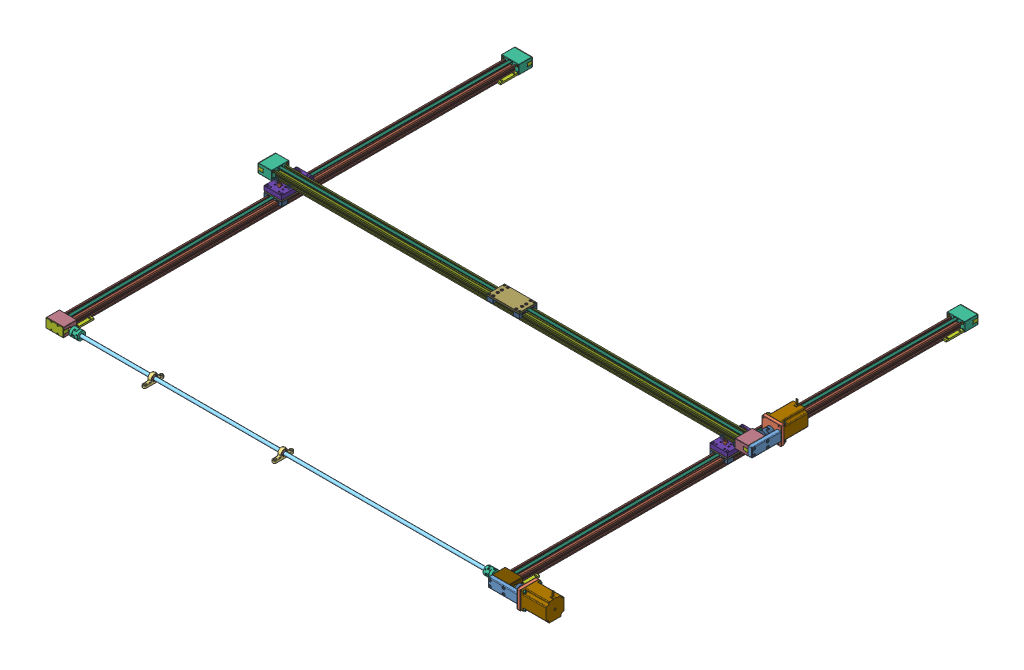
SolidWorks assembly 3390000-200221, configuration Default. Lengths in mm.
Overall size (1590.4 190.6 1456.62).
279 component instances, 43 part files, 6 mates.
Components (placement in the parent):
- 3390000-200221.stp-1: 3390000-200221.stp [Default] at origin size (1590.4 190.6 1456.62)
  - ZLW-0630S-G0BW0-D0A3C-AH2A0AE-1261.stp-1: ZLW-0630S-G0BW0-D0A3C-AH2A0AE-1261.stp [Default] at origin size (202.33 143.8 1456.02)
    - ZTL-063002.stp-1: ZTL-063002.stp [Default] at (15 -5.5 8) x (-1 0 0) z (0 0 -1) size (54 34.23 43)
      - ZTL-06300S-V.stp-1: ZTL-06300S-V.stp [Default] at (0 0 22) x (0 0.983968 0.178348) z (1 0 0) size (29.12 31.26 50)
        - ZTY-063002.stp-1: ZTY-063002.stp [Default] at origin size (20 20 49)
        - ZTY-063013.stp-1: ZTY-063013.stp [Default] at (0 0 20) x (-0.983968 0.178348 0) z (0 0 -1) size (24 24 12.01)
        - ZTY-063013.stp-2: ZTY-063013.stp [Default] at (0 0 -20) x (0.983968 -0.178348 0) z (0 0 1) size (24 24 12.01)
        - NOR-20902.stp-1: NOR-20902.stp [Default] at (0 0 13) x (0.345491 -0.938422 0) z (0 0 1) size (22 22 6)
        - NOR-20902.stp-2: NOR-20902.stp [Default] at (0 0 -13) x (-0.413146 -0.910665 0) z (0 0 -1) size (22 22 6)
        - NOR-10606.stp-1: NOR-10606.stp [Default] at (-10.5039 -10.2917 21.5) x (0.178348 0.983968 0) z (0 0 1) size (12.8 7 7)
        - NOR-10404.stp-1: NOR-10404.stp [Default] at (-7.2936 7.4198 21.5) x (0.178348 0.983968 0) z (0 0 1) size (6 4 4)
        - NOR-10606.stp-2: NOR-10606.stp [Default] at (6.2236 -13.3236 21.5) x (0.178348 0.983968 0) z (0 0 1) size (12.8 7 7)
        - NOR-10404.stp-2: NOR-10404.stp [Default] at (9.4338 4.3878 21.5) x (0.178348 0.983968 0) z (0 0 1) size (6 4 4)
        - NOR-10606.stp-3: NOR-10606.stp [Default] at (-10.5039 -10.2917 -21.5) x (0.178348 0.983968 0) z (0 0 1) size (12.8 7 7)
        - NOR-10404.stp-3: NOR-10404.stp [Default] at (-7.2936 7.4198 -21.5) x (0.178348 0.983968 0) z (0 0 1) size (6 4 4)
        - NOR-10606.stp-4: NOR-10606.stp [Default] at (6.2236 -13.3236 -21.5) x (0.178348 0.983968 0) z (0 0 1) size (12.8 7 7)
        - NOR-10404.stp-4: NOR-10404.stp [Default] at (9.4338 4.3878 -21.5) x (0.178348 0.983968 0) z (0 0 1) size (6 4 4)
      - ZTZ-063001.stp-1: ZTZ-063001.stp [Default] at origin size (54 28 40)
      - ZTZ-063002.stp-1: ZTZ-063002.stp [Default] at (0 0 40) size (54 28 17.34)
      - NOR-20110.stp-1: NOR-20110.stp [Default] at (-10 0 5) size (6 6 8.5)
      - NOR-20110.stp-2: NOR-20110.stp [Default] at (10 0 5) size (6 6 8.5)
      - ZTZ-063009.stp-1: ZTZ-063009.stp [Default] at (-21.5 8.5 -1) size (6 6 7)
      - ZTZ-063009.stp-2: ZTZ-063009.stp [Default] at (21.5 8.5 -1) size (6 6 7)
    - ZS-063003.stp-1: ZS-063003.stp [Default] at (15 11.5 688.5) size (54.46 17.5 100)
      - WJ200QM-01-06.stp-1: WJ200QM-01-06.stp [Default] at (-15 -11.5 40.5) size (18 12.5 19.01)
        - WM-01-06.stp-1: WM-01-06.stp [Default] at origin size (18 12.5 19.01)
        - J200QM-01-06.stp-1: J200QM-01-06.stp [Default] at origin size (8.77 8.77 19)
      - WJ200QM-01-06.stp-2: WJ200QM-01-06.stp [Default] at (-15 -11.5 -40.5) size (18 12.5 19.01)
        - WM-01-06.stp-1: WM-01-06.stp [Default] at origin size (18 12.5 19.01)
        - J200QM-01-06.stp-1: J200QM-01-06.stp [Default] at origin size (8.77 8.77 19)
      - WJ200QM-01-06.stp-3: WJ200QM-01-06.stp [Default] at (15 -11.5 40.5) x (-1 0 0) z (0 0 -1) size (18 12.5 19.01)
        - WM-01-06.stp-1: WM-01-06.stp [Default] at origin size (18 12.5 19.01)
        - J200QM-01-06.stp-1: J200QM-01-06.stp [Default] at origin size (8.77 8.77 19)
      - WJ200QM-01-06.stp-4: WJ200QM-01-06.stp [Default] at (15 -11.5 -40.5) x (-1 0 0) z (0 0 -1) size (18 12.5 19.01)
        - WM-01-06.stp-1: WM-01-06.stp [Default] at origin size (18 12.5 19.01)
        - J200QM-01-06.stp-1: J200QM-01-06.stp [Default] at origin size (8.77 8.77 19)
      - ZSY-063005.stp-1: ZSY-063005.stp [Default] at origin size (54 5 100)
      - NOR-10606_1.stp-1: NOR-10606_1.stp [Default] at (-22.5 -3 -35.5) x (0 -1 0) z (0.884514 0 -0.466514) size (12.8 7 7)
      - NOR-10606_1.stp-2: NOR-10606_1.stp [Default] at (-22.5 -3 35.5) x (0 -1 0) z (0.884514 0 -0.466514) size (12.8 7 7)
      - NOR-10606_1.stp-3: NOR-10606_1.stp [Default] at (22.5 -3 -35.5) x (0 -1 0) z (0.884514 0 -0.466514) size (12.8 7 7)
      - NOR-10606_1.stp-4: NOR-10606_1.stp [Default] at (22.5 -3 35.5) x (0 -1 0) z (0.884514 0 -0.466514) size (12.8 7 7)
    - ZR-063002.stp-1: ZR-063002.stp [Default] at (-41.9573 -64.3073 568.8616) x (0.000555 -0.999099 0.042429) z (0.034715 0.042422 0.998496) size (83.45 58.44 1423.14)
      - ZSY-063002.stp-1: ZSY-063002.stp [Default] at (-64.7242 63.004 87.2023) x (0.042429 -0.034707 0.998496) z (-0.000555 -0.999397 -0.034715) size (25 5.02 18)
      - ZSY-063002.stp-2: ZSY-063002.stp [Default] at (-61.552 42.4118 161.4647) x (-0.042429 0.034707 -0.998496) z (0.000555 0.999397 0.034715) size (25 5.02 18)
      - ZR-063002-XX.stp-1: ZR-063002-XX.stp [Default] at (-53.6573 52.7253 123.6809) x (0.042429 -0.034707 0.998496) z (-0.000555 -0.999397 -0.034715) size (1423.99 23.05 9.01)
      - NOR-10606_1.stp-1: NOR-10606_1.stp [Default] at (-66.0394 57.8983 162.1937) x (0.999099 0.000918 -0.042422) z (0.042422 0.000019 0.9991) size (12.8 7 7)
      - NOR-10606_1.stp-2: NOR-10606_1.stp [Default] at (-66.0466 44.9062 161.7424) x (0.999099 0.000918 -0.042422) z (0.042431 -0.013069 0.999014) size (12.8 7 7)
      - NOR-10606_1.stp-3: NOR-10606_1.stp [Default] at (-69.2215 60.5014 87.3065) x (0.999099 0.000918 -0.042422) z (0.042431 -0.013069 0.999014) size (12.8 7 7)
      - NOR-10606_1.stp-4: NOR-10606_1.stp [Default] at (-69.2287 47.5092 86.8552) x (0.999099 0.000918 -0.042422) z (0.042431 -0.013069 0.999014) size (12.8 7 7)
    - ZTF-063006.stp-1: ZTF-063006.stp [Default] at (15 -5.5 1369) size (93 32.42 42)
      - ZTF-06300S-R-L-V.stp-1: ZTF-06300S-R-L-V.stp [Default] at (-16.9444 -7.7633 33.6167) x (0 -0.983968 0.178348) z (-1 0 0) size (27.9 27.9 93)
        - Antriebswelle-beidseitig.stp-1: Antriebswelle-beidseitig.stp [Default] at (-9.7106 -10.0459 -63.4444) x (0.996733 -0.080762 0) z (0 0 1) size (22.49 22.49 93)
          - Welle-beidseitig.stp-1: Welle-beidseitig.stp [Default] at origin size (12 12 93)
          - riemenrad.stp-1: riemenrad.stp [Default] at (0 0 45.5) x (0.99106 -0.133414 0) z (0 0 1) size (20 20 11.8)
        - NOR-20902.stp-1: NOR-20902.stp [Default] at (-9.7106 -10.0459 -3.9444) size (22 22 6)
        - NOR-20902.stp-2: NOR-20902.stp [Default] at (-9.7106 -10.0459 -29.9444) x (1 0 0) z (0 0 -1) size (22 22 6)
        - ZTY-063013.stp-1: ZTY-063013.stp [Default] at (-9.7106 -10.0459 3.0556) x (-0.983968 0.178348 0) z (0 0 -1) size (24 24 12.01)
        - ZTY-063013.stp-2: ZTY-063013.stp [Default] at (-9.7106 -10.0459 -36.9444) x (0.983968 -0.178348 0) z (0 0 1) size (24 24 12.01)
      - ZTZ-063005.stp-1: ZTZ-063005.stp [Default] at origin size (54 28 40)
      - ZTZ-063002.stp-1: ZTZ-063002.stp [Default] at (0 0 40) size (54 28 17.34)
      - NOR-20110.stp-1: NOR-20110.stp [Default] at (-10 0 5) size (6 6 8.5)
      - NOR-20110.stp-2: NOR-20110.stp [Default] at (10 0 5) size (6 6 8.5)
    - MK-0070.stp-1: MK-0070.stp [Default] at (87.4 -5.5 1391) x (-1 0 0) z (0 0 1) size (175.4 74.4 60.41)
      - MF-0630-NEMA23-S.stp-1: MF-0630-NEMA23-S.stp [Default] at origin size (109.2 57.6 60.41)
        - ZTY-063027.stp-1: ZTY-063027.stp [Default] at (32.4 0 12) x (-1 0 0) z (0 0 1) size (89.4 28 19.02)
        - ZTY-063006.stp-1: ZTY-063006.stp [Default] x (0 -1 0) z (1 0 0) size (56.4 59 10.03)
        - MH-06.stp-1: MH-06.stp [Default] at (12.4 8 25) x (0 -0.79027 0.612759) z (0 0.612759 0.79027) size (8 9.2 8)
        - MH-06.stp-2: MH-06.stp [Default] at (12.4 -8 25) x (0 -0.506668 -0.862141) z (0 0.862141 -0.506668) size (8 9.2 8)
        - NOR-10517.stp-1: NOR-10517.stp [Default] at (6 -8 25) size (26 10 10)
        - NOR-10517.stp-2: NOR-10517.stp [Default] at (6 8 25) size (26 10 10)
        - NOR-10520.stp-1: NOR-10520.stp [Default] at (93.75 8.5 26) x (0 0 -1) z (1 0 0) size (29 7 7)
        - NOR-10520.stp-2: NOR-10520.stp [Default] at (51.25 8.5 26) x (0 0 -1) z (1 0 0) size (29 7 7)
        - NOR-10520.stp-3: NOR-10520.stp [Default] at (93.75 -8.5 26) x (0 0 -1) z (1 0 0) size (29 7 7)
        - NOR-10520.stp-4: NOR-10520.stp [Default] at (51.25 -8.5 26) x (0 0 -1) z (1 0 0) size (29 7 7)
        - NOR-10523.stp-1: NOR-10523.stp [Default] at (-5.8 -23.57 23.57) x (1 0 0) z (0 -0.947418 0.319998) size (20 7 7)
        - NOR-10523.stp-2: NOR-10523.stp [Default] at (-5.8 23.57 -23.57) x (1 0 0) z (0 0.8789 -0.477006) size (20 7 7)
        - NOR-10523.stp-3: NOR-10523.stp [Default] at (-5.8 -23.57 -23.57) x (1 0 0) z (0 0.932913 0.360102) size (20 7 7)
        - NOR-10523.stp-4: NOR-10523.stp [Default] at (-5.8 23.57 23.57) x (1 0 0) z (0 0.637688 0.770295) size (20 7 7)
        - NOR-11003.stp-1: NOR-11003.stp [Default] at (-5 23.57 -23.57) x (-1 0 0) z (0 0.362571 -0.931956) size (0.8 9 9)
        - NOR-11003.stp-2: NOR-11003.stp [Default] at (-5 23.57 23.57) x (-1 0 0) z (0 0 -1) size (0.8 9 9)
        - NOR-11003.stp-3: NOR-11003.stp [Default] at (-5 -23.57 -23.57) x (-1 0 0) z (0 0 -1) size (0.8 9 9)
        - NOR-11003.stp-4: NOR-11003.stp [Default] at (-5 -23.57 23.57) x (-1 0 0) z (0 0 -1) size (0.8 9 9)
        - ZSG.stp-1: ZSG.stp [Default] at (51.25 0 6) x (0 0 1) z (0.488795 -0.872398 0) size (8 3 3)
        - ZSG.stp-2: ZSG.stp [Default] at (93.75 0 6) x (0 0 1) z (-1 0 0) size (8 3 3)
      - MOT-AN-S-060-020-056-L-A-AAAA.stp-1: MOT-AN-S-060-020-056-L-A-AAAA.stp [Default] x (0 0 -1) z (1 0 0) size (56.4 73.2 96.6)
      - COU-AR-K-063-080-25-26-B-AAAA.stp-1: COU-AR-K-063-080-25-26-B-AAAA.stp [Default] at (23.75 0 0) x (0 0.270836 0.962626) z (-1 0 0) size (25.21 25.21 25.5)
    - ZSX-063001.stp-1: ZSX-063001.stp [Default] at origin size (35 22 1377)
  - ZLW-0630S-G0BW0-D0A1C-0A0A0-1261.stp-1: ZLW-0630S-G0BW0-D0A1C-0A0A0-1261.stp [Default] at (-1373 0 0) size (107.86 143.8 1445)
    - ZTL-063002.stp-1: ZTL-063002.stp [Default] at (15 -5.5 8) x (-1 0 0) z (0 0 -1) size (54 34.23 43)
      - ZTL-06300S-V.stp-1: ZTL-06300S-V.stp [Default] at (0 0 22) x (0 0.983968 0.178348) z (1 0 0) size (29.12 31.26 50)
        - ZTY-063002.stp-1: ZTY-063002.stp [Default] at origin size (20 20 49)
        - ZTY-063013.stp-1: ZTY-063013.stp [Default] at (0 0 20) x (-0.983968 0.178348 0) z (0 0 -1) size (24 24 12.01)
        - ZTY-063013.stp-2: ZTY-063013.stp [Default] at (0 0 -20) x (0.983968 -0.178348 0) z (0 0 1) size (24 24 12.01)
        - NOR-20902.stp-1: NOR-20902.stp [Default] at (0 0 13) x (0.345491 -0.938422 0) z (0 0 1) size (22 22 6)
        - NOR-20902.stp-2: NOR-20902.stp [Default] at (0 0 -13) x (-0.413146 -0.910665 0) z (0 0 -1) size (22 22 6)
        - NOR-10606.stp-1: NOR-10606.stp [Default] at (-10.5039 -10.2917 21.5) x (0.178348 0.983968 0) z (0 0 1) size (12.8 7 7)
        - NOR-10404.stp-1: NOR-10404.stp [Default] at (-7.2936 7.4198 21.5) x (0.178348 0.983968 0) z (0 0 1) size (6 4 4)
        - NOR-10606.stp-2: NOR-10606.stp [Default] at (6.2236 -13.3236 21.5) x (0.178348 0.983968 0) z (0 0 1) size (12.8 7 7)
        - NOR-10404.stp-2: NOR-10404.stp [Default] at (9.4338 4.3878 21.5) x (0.178348 0.983968 0) z (0 0 1) size (6 4 4)
        - NOR-10606.stp-3: NOR-10606.stp [Default] at (-10.5039 -10.2917 -21.5) x (0.178348 0.983968 0) z (0 0 1) size (12.8 7 7)
        - NOR-10404.stp-3: NOR-10404.stp [Default] at (-7.2936 7.4198 -21.5) x (0.178348 0.983968 0) z (0 0 1) size (6 4 4)
        - NOR-10606.stp-4: NOR-10606.stp [Default] at (6.2236 -13.3236 -21.5) x (0.178348 0.983968 0) z (0 0 1) size (12.8 7 7)
        - NOR-10404.stp-4: NOR-10404.stp [Default] at (9.4338 4.3878 -21.5) x (0.178348 0.983968 0) z (0 0 1) size (6 4 4)
      - ZTZ-063001.stp-1: ZTZ-063001.stp [Default] at origin size (54 28 40)
      - ZTZ-063002.stp-1: ZTZ-063002.stp [Default] at (0 0 40) size (54 28 17.34)
      - NOR-20110.stp-1: NOR-20110.stp [Default] at (-10 0 5) size (6 6 8.5)
      - NOR-20110.stp-2: NOR-20110.stp [Default] at (10 0 5) size (6 6 8.5)
      - ZTZ-063009.stp-1: ZTZ-063009.stp [Default] at (-21.5 8.5 -1) size (6 6 7)
      - ZTZ-063009.stp-2: ZTZ-063009.stp [Default] at (21.5 8.5 -1) size (6 6 7)
    - ZS-063003.stp-1: ZS-063003.stp [Default] at (15 11.5 688.5) size (54.46 17.5 100)
      - WJ200QM-01-06.stp-1: WJ200QM-01-06.stp [Default] at (-15 -11.5 40.5) size (18 12.5 19.01)
        - WM-01-06.stp-1: WM-01-06.stp [Default] at origin size (18 12.5 19.01)
        - J200QM-01-06.stp-1: J200QM-01-06.stp [Default] at origin size (8.77 8.77 19)
      - WJ200QM-01-06.stp-2: WJ200QM-01-06.stp [Default] at (-15 -11.5 -40.5) size (18 12.5 19.01)
        - WM-01-06.stp-1: WM-01-06.stp [Default] at origin size (18 12.5 19.01)
        - J200QM-01-06.stp-1: J200QM-01-06.stp [Default] at origin size (8.77 8.77 19)
      - WJ200QM-01-06.stp-3: WJ200QM-01-06.stp [Default] at (15 -11.5 40.5) x (-1 0 0) z (0 0 -1) size (18 12.5 19.01)
        - WM-01-06.stp-1: WM-01-06.stp [Default] at origin size (18 12.5 19.01)
        - J200QM-01-06.stp-1: J200QM-01-06.stp [Default] at origin size (8.77 8.77 19)
      - WJ200QM-01-06.stp-4: WJ200QM-01-06.stp [Default] at (15 -11.5 -40.5) x (-1 0 0) z (0 0 -1) size (18 12.5 19.01)
        - WM-01-06.stp-1: WM-01-06.stp [Default] at origin size (18 12.5 19.01)
        - J200QM-01-06.stp-1: J200QM-01-06.stp [Default] at origin size (8.77 8.77 19)
      - ZSY-063005.stp-1: ZSY-063005.stp [Default] at origin size (54 5 100)
      - NOR-10606_1.stp-1: NOR-10606_1.stp [Default] at (-22.5 -3 -35.5) x (0 -1 0) z (0.884514 0 -0.466514) size (12.8 7 7)
      - NOR-10606_1.stp-2: NOR-10606_1.stp [Default] at (-22.5 -3 35.5) x (0 -1 0) z (0.884514 0 -0.466514) size (12.8 7 7)
      - NOR-10606_1.stp-3: NOR-10606_1.stp [Default] at (22.5 -3 -35.5) x (0 -1 0) z (0.884514 0 -0.466514) size (12.8 7 7)
      - NOR-10606_1.stp-4: NOR-10606_1.stp [Default] at (22.5 -3 35.5) x (0 -1 0) z (0.884514 0 -0.466514) size (12.8 7 7)
    - ZR-063002.stp-1: ZR-063002.stp [Default] at (-41.9573 -64.3073 568.8616) x (0.000555 -0.999099 0.042429) z (0.034715 0.042422 0.998496) size (83.45 58.44 1423.14)
      - ZSY-063002.stp-1: ZSY-063002.stp [Default] at (-64.7242 63.004 87.2023) x (0.042429 -0.034707 0.998496) z (-0.000555 -0.999397 -0.034715) size (25 5.02 18)
      - ZSY-063002.stp-2: ZSY-063002.stp [Default] at (-61.552 42.4118 161.4647) x (-0.042429 0.034707 -0.998496) z (0.000555 0.999397 0.034715) size (25 5.02 18)
      - ZR-063002-XX.stp-1: ZR-063002-XX.stp [Default] at (-53.6573 52.7253 123.6809) x (0.042429 -0.034707 0.998496) z (-0.000555 -0.999397 -0.034715) size (1423.99 23.05 9.01)
      - NOR-10606_1.stp-1: NOR-10606_1.stp [Default] at (-66.0394 57.8983 162.1937) x (0.999099 0.000918 -0.042422) z (0.042422 0.000019 0.9991) size (12.8 7 7)
      - NOR-10606_1.stp-2: NOR-10606_1.stp [Default] at (-66.0466 44.9062 161.7424) x (0.999099 0.000918 -0.042422) z (0.042431 -0.013069 0.999014) size (12.8 7 7)
      - NOR-10606_1.stp-3: NOR-10606_1.stp [Default] at (-69.2215 60.5014 87.3065) x (0.999099 0.000918 -0.042422) z (0.042431 -0.013069 0.999014) size (12.8 7 7)
      - NOR-10606_1.stp-4: NOR-10606_1.stp [Default] at (-69.2287 47.5092 86.8552) x (0.999099 0.000918 -0.042422) z (0.042431 -0.013069 0.999014) size (12.8 7 7)
    - ZTF-063002.stp-1: ZTF-063002.stp [Default] at (15 -5.5 1369) size (73.5 30.97 44.8)
      - ZTF-06300S-V.stp-1: ZTF-06300S-V.stp [Default] at (0.1 0 22) x (0 -1 0) z (1 0 0) size (30.97 30.97 71.5)
        - ZTY-063003.stp-1: ZTY-063003.stp [Default] at origin size (20 20 70.8)
        - ZTY-063013.stp-1: ZTY-063013.stp [Default] at (0 0 19.9) x (1 0 0) z (0 0 -1) size (24 24 12.01)
        - ZTY-063013.stp-2: ZTY-063013.stp [Default] at (0 0 -20.1) x (-1 0 0) z (0 0 1) size (24 24 12.01)
        - NOR-20902.stp-1: NOR-20902.stp [Default] at (0 0 12.9) x (0.99266 -0.120936 0) z (0 0 1) size (22 22 6)
        - NOR-20902.stp-2: NOR-20902.stp [Default] at (0 0 -13.1) x (0.635824 -0.771834 0) z (0 0 -1) size (22 22 6)
      - ZTZ-063004.stp-1: ZTZ-063004.stp [Default] at origin size (54 28 40)
      - ZTZ-063002.stp-1: ZTZ-063002.stp [Default] at (0 0 40) size (54 28 17.34)
      - ZTZ-063009.stp-1: ZTZ-063009.stp [Default] at (21.5 8.5 -1) size (6 6 7)
      - ZTZ-063009.stp-2: ZTZ-063009.stp [Default] at (-21.5 8.5 -1) size (6 6 7)
      - NOR-20110.stp-1: NOR-20110.stp [Default] at (10 0 5) x (0.132077 0.991239 0) z (0 0 1) size (6 6 8.5)
      - NOR-20110.stp-2: NOR-20110.stp [Default] at (-10 0 5) x (-0.993719 0.111904 0) z (0 0 1) size (6 6 8.5)
      - NOR-10614.stp-1: NOR-10614.stp [Default] at (-21.5 -8.5 0) x (0 0 1) z (0.997351 -0.072733 0) size (18.8 7 7)
      - NOR-10614.stp-2: NOR-10614.stp [Default] at (21.5 -8.5 0) x (0 0 1) z (0.143912 0.98959 0) size (18.8 7 7)
    - ZSX-063001.stp-1: ZSX-063001.stp [Default] at origin size (35 22 1377)
  - ZLW-0630S-G0BW0-D0A1C-AH2A0AA-1327.stp-1: ZLW-0630S-G0BW0-D0A1C-AH2A0AA-1327.stp [Default] at (-1393 44 703.5) x (0 0 -1) z (1 0 0) size (204.62 149.4 1522.02)
    - ZTL-063002.stp-1: ZTL-063002.stp [Default] at (15 -5.5 8) x (-1 0 0) z (0 0 -1) size (54 34.23 43)
      - ZTL-06300S-V.stp-1: ZTL-06300S-V.stp [Default] at (0 0 22) x (0 0.983968 0.178348) z (1 0 0) size (29.12 31.26 50)
        - ZTY-063002.stp-1: ZTY-063002.stp [Default] at origin size (20 20 49)
        - ZTY-063013.stp-1: ZTY-063013.stp [Default] at (0 0 20) x (-0.983968 0.178348 0) z (0 0 -1) size (24 24 12.01)
        - ZTY-063013.stp-2: ZTY-063013.stp [Default] at (0 0 -20) x (0.983968 -0.178348 0) z (0 0 1) size (24 24 12.01)
        - NOR-20902.stp-1: NOR-20902.stp [Default] at (0 0 13) x (0.345491 -0.938422 0) z (0 0 1) size (22 22 6)
        - NOR-20902.stp-2: NOR-20902.stp [Default] at (0 0 -13) x (-0.413146 -0.910665 0) z (0 0 -1) size (22 22 6)
        - NOR-10606.stp-1: NOR-10606.stp [Default] at (-10.5039 -10.2917 21.5) x (0.178348 0.983968 0) z (0 0 1) size (12.8 7 7)
        - NOR-10404.stp-1: NOR-10404.stp [Default] at (-7.2936 7.4198 21.5) x (0.178348 0.983968 0) z (0 0 1) size (6 4 4)
        - NOR-10606.stp-2: NOR-10606.stp [Default] at (6.2236 -13.3236 21.5) x (0.178348 0.983968 0) z (0 0 1) size (12.8 7 7)
        - NOR-10404.stp-2: NOR-10404.stp [Default] at (9.4338 4.3878 21.5) x (0.178348 0.983968 0) z (0 0 1) size (6 4 4)
        - NOR-10606.stp-3: NOR-10606.stp [Default] at (-10.5039 -10.2917 -21.5) x (0.178348 0.983968 0) z (0 0 1) size (12.8 7 7)
        - NOR-10404.stp-3: NOR-10404.stp [Default] at (-7.2936 7.4198 -21.5) x (0.178348 0.983968 0) z (0 0 1) size (6 4 4)
        - NOR-10606.stp-4: NOR-10606.stp [Default] at (6.2236 -13.3236 -21.5) x (0.178348 0.983968 0) z (0 0 1) size (12.8 7 7)
        - NOR-10404.stp-4: NOR-10404.stp [Default] at (9.4338 4.3878 -21.5) x (0.178348 0.983968 0) z (0 0 1) size (6 4 4)
      - ZTZ-063001.stp-1: ZTZ-063001.stp [Default] at origin size (54 28 40)
      - ZTZ-063002.stp-1: ZTZ-063002.stp [Default] at (0 0 40) size (54 28 17.34)
      - NOR-20110.stp-1: NOR-20110.stp [Default] at (-10 0 5) size (6 6 8.5)
      - NOR-20110.stp-2: NOR-20110.stp [Default] at (10 0 5) size (6 6 8.5)
      - ZTZ-063009.stp-1: ZTZ-063009.stp [Default] at (-21.5 8.5 -1) size (6 6 7)
      - ZTZ-063009.stp-2: ZTZ-063009.stp [Default] at (21.5 8.5 -1) size (6 6 7)
    - ZS-063003.stp-1: ZS-063003.stp [Default] at (15 11.5 721.5) size (54.46 17.5 100)
      - WJ200QM-01-06.stp-1: WJ200QM-01-06.stp [Default] at (-15 -11.5 40.5) size (18 12.5 19.01)
        - WM-01-06.stp-1: WM-01-06.stp [Default] at origin size (18 12.5 19.01)
        - J200QM-01-06.stp-1: J200QM-01-06.stp [Default] at origin size (8.77 8.77 19)
      - WJ200QM-01-06.stp-2: WJ200QM-01-06.stp [Default] at (-15 -11.5 -40.5) size (18 12.5 19.01)
        - WM-01-06.stp-1: WM-01-06.stp [Default] at origin size (18 12.5 19.01)
        - J200QM-01-06.stp-1: J200QM-01-06.stp [Default] at origin size (8.77 8.77 19)
      - WJ200QM-01-06.stp-3: WJ200QM-01-06.stp [Default] at (15 -11.5 40.5) x (-1 0 0) z (0 0 -1) size (18 12.5 19.01)
        - WM-01-06.stp-1: WM-01-06.stp [Default] at origin size (18 12.5 19.01)
        - J200QM-01-06.stp-1: J200QM-01-06.stp [Default] at origin size (8.77 8.77 19)
      - WJ200QM-01-06.stp-4: WJ200QM-01-06.stp [Default] at (15 -11.5 -40.5) x (-1 0 0) z (0 0 -1) size (18 12.5 19.01)
        - WM-01-06.stp-1: WM-01-06.stp [Default] at origin size (18 12.5 19.01)
        - J200QM-01-06.stp-1: J200QM-01-06.stp [Default] at origin size (8.77 8.77 19)
      - ZSY-063005.stp-1: ZSY-063005.stp [Default] at origin size (54 5 100)
      - NOR-10606_1.stp-1: NOR-10606_1.stp [Default] at (-22.5 -3 -35.5) x (0 -1 0) z (0.884514 0 -0.466514) size (12.8 7 7)
      - NOR-10606_1.stp-2: NOR-10606_1.stp [Default] at (-22.5 -3 35.5) x (0 -1 0) z (0.884514 0 -0.466514) size (12.8 7 7)
      - NOR-10606_1.stp-3: NOR-10606_1.stp [Default] at (22.5 -3 -35.5) x (0 -1 0) z (0.884514 0 -0.466514) size (12.8 7 7)
      - NOR-10606_1.stp-4: NOR-10606_1.stp [Default] at (22.5 -3 35.5) x (0 -1 0) z (0.884514 0 -0.466514) size (12.8 7 7)
    - ZR-063002_1.stp-1: ZR-063002_1.stp [Default] at (-41.9573 -64.3073 601.8616) x (0.000555 -0.999099 0.042429) z (0.034715 0.042422 0.998496) size (86.25 60.73 1489.04)
      - ZSY-063002.stp-1: ZSY-063002.stp [Default] at (-64.7242 63.004 87.2023) x (0.042429 -0.034707 0.998496) z (-0.000555 -0.999397 -0.034715) size (25 5.02 18)
      - ZSY-063002.stp-2: ZSY-063002.stp [Default] at (-61.552 42.4118 161.4647) x (-0.042429 0.034707 -0.998496) z (0.000555 0.999397 0.034715) size (25 5.02 18)
      - ZR-063002-XX_1.stp-1: ZR-063002-XX_1.stp [Default] at (-53.6573 52.7253 123.6809) x (0.042429 -0.034707 0.998496) z (-0.000555 -0.999397 -0.034715) size (1489.99 23.05 9.01)
      - NOR-10606_1.stp-1: NOR-10606_1.stp [Default] at (-66.0394 57.8983 162.1937) x (0.999099 0.000918 -0.042422) z (0.042422 0.000019 0.9991) size (12.8 7 7)
      - NOR-10606_1.stp-2: NOR-10606_1.stp [Default] at (-66.0466 44.9062 161.7424) x (0.999099 0.000918 -0.042422) z (0.042431 -0.013069 0.999014) size (12.8 7 7)
      - NOR-10606_1.stp-3: NOR-10606_1.stp [Default] at (-69.2215 60.5014 87.3065) x (0.999099 0.000918 -0.042422) z (0.042431 -0.013069 0.999014) size (12.8 7 7)
      - NOR-10606_1.stp-4: NOR-10606_1.stp [Default] at (-69.2287 47.5092 86.8552) x (0.999099 0.000918 -0.042422) z (0.042431 -0.013069 0.999014) size (12.8 7 7)
    - ZTF-063002.stp-1: ZTF-063002.stp [Default] at (15 -5.5 1435) size (73.5 30.97 44.8)
      - ZTF-06300S-V.stp-1: ZTF-06300S-V.stp [Default] at (0.1 0 22) x (0 -1 0) z (1 0 0) size (30.97 30.97 71.5)
        - ZTY-063003.stp-1: ZTY-063003.stp [Default] at origin size (20 20 70.8)
        - ZTY-063013.stp-1: ZTY-063013.stp [Default] at (0 0 19.9) x (1 0 0) z (0 0 -1) size (24 24 12.01)
        - ZTY-063013.stp-2: ZTY-063013.stp [Default] at (0 0 -20.1) x (-1 0 0) z (0 0 1) size (24 24 12.01)
        - NOR-20902.stp-1: NOR-20902.stp [Default] at (0 0 12.9) x (0.99266 -0.120936 0) z (0 0 1) size (22 22 6)
        - NOR-20902.stp-2: NOR-20902.stp [Default] at (0 0 -13.1) x (0.635824 -0.771834 0) z (0 0 -1) size (22 22 6)
      - ZTZ-063004.stp-1: ZTZ-063004.stp [Default] at origin size (54 28 40)
      - ZTZ-063002.stp-1: ZTZ-063002.stp [Default] at (0 0 40) size (54 28 17.34)
      - ZTZ-063009.stp-1: ZTZ-063009.stp [Default] at (21.5 8.5 -1) size (6 6 7)
      - ZTZ-063009.stp-2: ZTZ-063009.stp [Default] at (-21.5 8.5 -1) size (6 6 7)
      - NOR-20110.stp-1: NOR-20110.stp [Default] at (10 0 5) x (0.132077 0.991239 0) z (0 0 1) size (6 6 8.5)
      - NOR-20110.stp-2: NOR-20110.stp [Default] at (-10 0 5) x (-0.993719 0.111904 0) z (0 0 1) size (6 6 8.5)
      - NOR-10614.stp-1: NOR-10614.stp [Default] at (-21.5 -8.5 0) x (0 0 1) z (0.997351 -0.072733 0) size (18.8 7 7)
      - NOR-10614.stp-2: NOR-10614.stp [Default] at (21.5 -8.5 0) x (0 0 1) z (0.143912 0.98959 0) size (18.8 7 7)
    - MK-0070.stp-1: MK-0070.stp [Default] at (87.4 -5.5 1457) x (-1 0 0) z (0 0 1) size (175.4 74.4 60.41)
      - MF-0630-NEMA23-S.stp-1: MF-0630-NEMA23-S.stp [Default] at origin size (109.2 57.6 60.41)
        - ZTY-063027.stp-1: ZTY-063027.stp [Default] at (32.4 0 12) x (-1 0 0) z (0 0 1) size (89.4 28 19.02)
        - ZTY-063006.stp-1: ZTY-063006.stp [Default] x (0 -1 0) z (1 0 0) size (56.4 59 10.03)
        - MH-06.stp-1: MH-06.stp [Default] at (12.4 8 25) x (0 -0.79027 0.612759) z (0 0.612759 0.79027) size (8 9.2 8)
        - MH-06.stp-2: MH-06.stp [Default] at (12.4 -8 25) x (0 -0.506668 -0.862141) z (0 0.862141 -0.506668) size (8 9.2 8)
        - NOR-10517.stp-1: NOR-10517.stp [Default] at (6 -8 25) size (26 10 10)
        - NOR-10517.stp-2: NOR-10517.stp [Default] at (6 8 25) size (26 10 10)
        - NOR-10520.stp-1: NOR-10520.stp [Default] at (93.75 8.5 26) x (0 0 -1) z (1 0 0) size (29 7 7)
        - NOR-10520.stp-2: NOR-10520.stp [Default] at (51.25 8.5 26) x (0 0 -1) z (1 0 0) size (29 7 7)
        - NOR-10520.stp-3: NOR-10520.stp [Default] at (93.75 -8.5 26) x (0 0 -1) z (1 0 0) size (29 7 7)
        - NOR-10520.stp-4: NOR-10520.stp [Default] at (51.25 -8.5 26) x (0 0 -1) z (1 0 0) size (29 7 7)
        - NOR-10523.stp-1: NOR-10523.stp [Default] at (-5.8 -23.57 23.57) x (1 0 0) z (0 -0.947418 0.319998) size (20 7 7)
        - NOR-10523.stp-2: NOR-10523.stp [Default] at (-5.8 23.57 -23.57) x (1 0 0) z (0 0.8789 -0.477006) size (20 7 7)
        - NOR-10523.stp-3: NOR-10523.stp [Default] at (-5.8 -23.57 -23.57) x (1 0 0) z (0 0.932913 0.360102) size (20 7 7)
        - NOR-10523.stp-4: NOR-10523.stp [Default] at (-5.8 23.57 23.57) x (1 0 0) z (0 0.637688 0.770295) size (20 7 7)
        - NOR-11003.stp-1: NOR-11003.stp [Default] at (-5 23.57 -23.57) x (-1 0 0) z (0 0.362571 -0.931956) size (0.8 9 9)
        - NOR-11003.stp-2: NOR-11003.stp [Default] at (-5 23.57 23.57) x (-1 0 0) z (0 0 -1) size (0.8 9 9)
        - NOR-11003.stp-3: NOR-11003.stp [Default] at (-5 -23.57 -23.57) x (-1 0 0) z (0 0 -1) size (0.8 9 9)
        - NOR-11003.stp-4: NOR-11003.stp [Default] at (-5 -23.57 23.57) x (-1 0 0) z (0 0 -1) size (0.8 9 9)
        - ZSG.stp-1: ZSG.stp [Default] at (51.25 0 6) x (0 0 1) z (0.488795 -0.872398 0) size (8 3 3)
        - ZSG.stp-2: ZSG.stp [Default] at (93.75 0 6) x (0 0 1) z (-1 0 0) size (8 3 3)
      - MOT-AN-S-060-020-056-L-A-AAAA.stp-1: MOT-AN-S-060-020-056-L-A-AAAA.stp [Default] x (0 0 -1) z (1 0 0) size (56.4 73.2 96.6)
      - COU-AR-K-063-080-25-26-B-AAAA.stp-1: COU-AR-K-063-080-25-26-B-AAAA.stp [Default] at (23.75 0 0) x (0 0.270836 0.962626) z (-1 0 0) size (25.21 25.21 25.5)
    - ZSX-063001_1.stp-1: ZSX-063001_1.stp [Default] at origin size (35 22 1443)
  - AK-0011.stp-1: AK-0011.stp [Default] at (-1358 11.5 688.5) x (1 0 0) z (0 1 0) size (1427 100 36)
    - ZWY-063004.stp-1: ZWY-063004.stp [Default] at origin size (54 100 13)
    - ZWY-063004.stp-2: ZWY-063004.stp [Default] at (1373 0 0) size (54 100 13)
    - NOR-10614_1.stp-1: NOR-10614_1.stp [Default] at (-22.5 -45.5 4) x (0 0 -1) z (1 0 0) size (18.8 7 7)
    - NOR-10614_1.stp-2: NOR-10614_1.stp [Default] at (1350.5 -45.5 4) x (0 0 -1) z (1 0 0) size (18.8 7 7)
    - NOR-10614_1.stp-3: NOR-10614_1.stp [Default] at (22.5 -45.5 4) x (0 0 -1) z (1 0 0) size (18.8 7 7)
    - NOR-10614_1.stp-4: NOR-10614_1.stp [Default] at (1395.5 -45.5 4) x (0 0 -1) z (1 0 0) size (18.8 7 7)
    - NOR-10614_1.stp-5: NOR-10614_1.stp [Default] at (-22.5 45.5 4) x (0 0 -1) z (1 0 0) size (18.8 7 7)
    - NOR-10614_1.stp-6: NOR-10614_1.stp [Default] at (1350.5 45.5 4) x (0 0 -1) z (1 0 0) size (18.8 7 7)
    - NOR-10614_1.stp-7: NOR-10614_1.stp [Default] at (22.5 45.5 4) x (0 0 -1) z (1 0 0) size (18.8 7 7)
    - NOR-10614_1.stp-8: NOR-10614_1.stp [Default] at (1395.5 45.5 4) x (0 0 -1) z (1 0 0) size (18.8 7 7)
    - NOR-10610.stp-1: NOR-10610.stp [Default] at (-19.5 -20 18) x (0 0 -1) z (1 0 0) size (15.5 8.5 8.5)
    - NOR-10610.stp-2: NOR-10610.stp [Default] at (1353.5 -20 18) x (0 0 -1) z (1 0 0) size (15.5 8.5 8.5)
    - NOR-10610.stp-3: NOR-10610.stp [Default] at (19.5 -20 18) x (0 0 -1) z (1 0 0) size (15.5 8.5 8.5)
    - NOR-10610.stp-4: NOR-10610.stp [Default] at (1392.5 -20 18) x (0 0 -1) z (1 0 0) size (15.5 8.5 8.5)
    - NOR-10610.stp-5: NOR-10610.stp [Default] at (-19.5 20 18) x (0 0 -1) z (1 0 0) size (15.5 8.5 8.5)
    - NOR-10610.stp-6: NOR-10610.stp [Default] at (1353.5 20 18) x (0 0 -1) z (1 0 0) size (15.5 8.5 8.5)
    - NOR-10610.stp-7: NOR-10610.stp [Default] at (19.5 20 18) x (0 0 -1) z (1 0 0) size (15.5 8.5 8.5)
    - NOR-10610.stp-8: NOR-10610.stp [Default] at (1392.5 20 18) x (0 0 -1) z (1 0 0) size (15.5 8.5 8.5)
    - NOR-10531.stp-1: NOR-10531.stp [Default] at (0 -30 18) x (0 0 -1) z (1 0 0) size (18 10 10)
    - NOR-10531.stp-2: NOR-10531.stp [Default] at (1373 -30 18) x (0 0 -1) z (1 0 0) size (18 10 10)
    - NOR-10531.stp-3: NOR-10531.stp [Default] at (0 30 18) x (0 0 -1) z (1 0 0) size (18 10 10)
    - NOR-10531.stp-4: NOR-10531.stp [Default] at (1373 30 18) x (0 0 -1) z (1 0 0) size (18 10 10)
  - KSTM-10.stp-1: KSTM-10.stp [Default] at (-1074.8332 -19.5 1391) x (0 0 -1) z (0 1 0) size (63.24 14 27.55)
    - E4use).stp-1: E4use).stp [Default] at origin size (63.24 13.02 27.55)
    - WKM-10-14.stp-1: WKM-10-14.stp [Default] at (0 0 14) size (19 14 19)
  - KSTM-10.stp-2: KSTM-10.stp [Default] at (-674.8332 -19.5 1391) x (0 0 -1) z (0 1 0) size (63.24 14 27.55)
    - E4use).stp-1: E4use).stp [Default] at origin size (63.24 13.02 27.55)
    - WKM-10-14.stp-1: WKM-10-14.stp [Default] at (0 0 14) size (19 14 19)
  - AWMP-10-1272.stp-1: AWMP-10-1272.stp [Default] at (-670.5 -5.5 1391) x (0 -0.934038 0.357174) z (1 0 0) size (10 10 1272)
  - COU-AR-K-080-100-25-26-B-AAAA.stp-1: COU-AR-K-080-100-25-26-B-AAAA.stp [Default] at (-32.75 -5.5 1391) x (0 -0.999042 0.043766) z (1 0 0) size (25.21 25.21 25.5)
  - COU-AR-K-080-100-25-26-B-AAAA.stp-2: COU-AR-K-080-100-25-26-B-AAAA.stp [Default] at (-1308.25 -5.5 1391) x (0 0.458834 -0.888522) z (-1 0 0) size (25.21 25.21 25.5)
- TEMPORARY_MountingBracket-1: TEMPORARY_MountingBracket [Default] at (35 -17 35) x (0 0 1) z (-1 0 0) size (54 5 10)
- TEMPORARY_MountingBracket-2: TEMPORARY_MountingBracket [Default] at (-5 -17 35) x (0 0 1) z (-1 0 0) size (54 5 10)
- TEMPORARY_MountingBracket-3: TEMPORARY_MountingBracket [Default] at (-1378 -17 35) x (0 0 1) z (-1 0 0) size (54 5 10)
- TEMPORARY_MountingBracket-4: TEMPORARY_MountingBracket [Default] at (-1338 -17 35) x (0 0 1) z (-1 0 0) size (54 5 10)
- TEMPORARY_MountingBracket-5: TEMPORARY_MountingBracket [Default] at (35 -17 1342) x (0 0 -1) z (1 0 0) size (54 5 10)
- TEMPORARY_MountingBracket-6: TEMPORARY_MountingBracket [Default] at (-5 -17 1342) x (0 0 -1) z (1 0 0) size (54 5 10)
- TEMPORARY_MountingBracket-7: TEMPORARY_MountingBracket [Default] at (-1378 -17 1342) x (0 0 -1) z (1 0 0) size (54 5 10)
- TEMPORARY_MountingBracket-8: TEMPORARY_MountingBracket [Default] at (-1338 -17 1342) x (0 0 -1) z (1 0 0) size (54 5 10)
Mates (geometry in assembly coordinates):
- Coincident1: coincident aligned: plane of 3390000-200221.stp-1/ZLW-0630S-G0BW0-D0A3C-AH2A0AE-1261.stp-1/ZTL-063002.stp-1/ZTZ-063001.stp-1 through (-12 -19.5 8) normal (0 -1 0); plane of TEMPORARY_MountingBracket-1 through (35 -19.5 35) normal (0 -1 0)
- Coincident2: coincident anti-aligned: plane of 3390000-200221.stp-1/ZLW-0630S-G0BW0-D0A3C-AH2A0AE-1261.stp-1/ZSX-063001.stp-1 through (30 -19.5 1377) normal (1 0 0); plane of TEMPORARY_MountingBracket-1 through (30 -19.5 8) normal (-1 0 0)
- Coincident3: coincident anti-aligned: plane of 3390000-200221.stp-1/ZLW-0630S-G0BW0-D0A3C-AH2A0AE-1261.stp-1/ZTL-063002.stp-1/ZTZ-063001.stp-1 through (15 -5.5 8) normal (0 0 1); plane of TEMPORARY_MountingBracket-1 through (40 -19.5 8) normal (0 0 -1)
- Coincident4: coincident aligned: plane of TEMPORARY_MountingBracket-1 through (35 -19.5 35) normal (0 -1 0); plane of TEMPORARY_MountingBracket-2 through (-5 -19.5 35) normal (0 -1 0)
- Coincident5: coincident anti-aligned: plane of 3390000-200221.stp-1/ZLW-0630S-G0BW0-D0A3C-AH2A0AE-1261.stp-1/ZSX-063001.stp-1 through (0 -15.15 1377) normal (-1 0 0); plane of TEMPORARY_MountingBracket-2 through (0 -19.5 8) normal (1 0 0)
- Coincident6: coincident aligned: plane of TEMPORARY_MountingBracket-1 through (35 -17 35) normal (0 0 1); plane of TEMPORARY_MountingBracket-2 through (-5 -17 35) normal (0 0 1)
